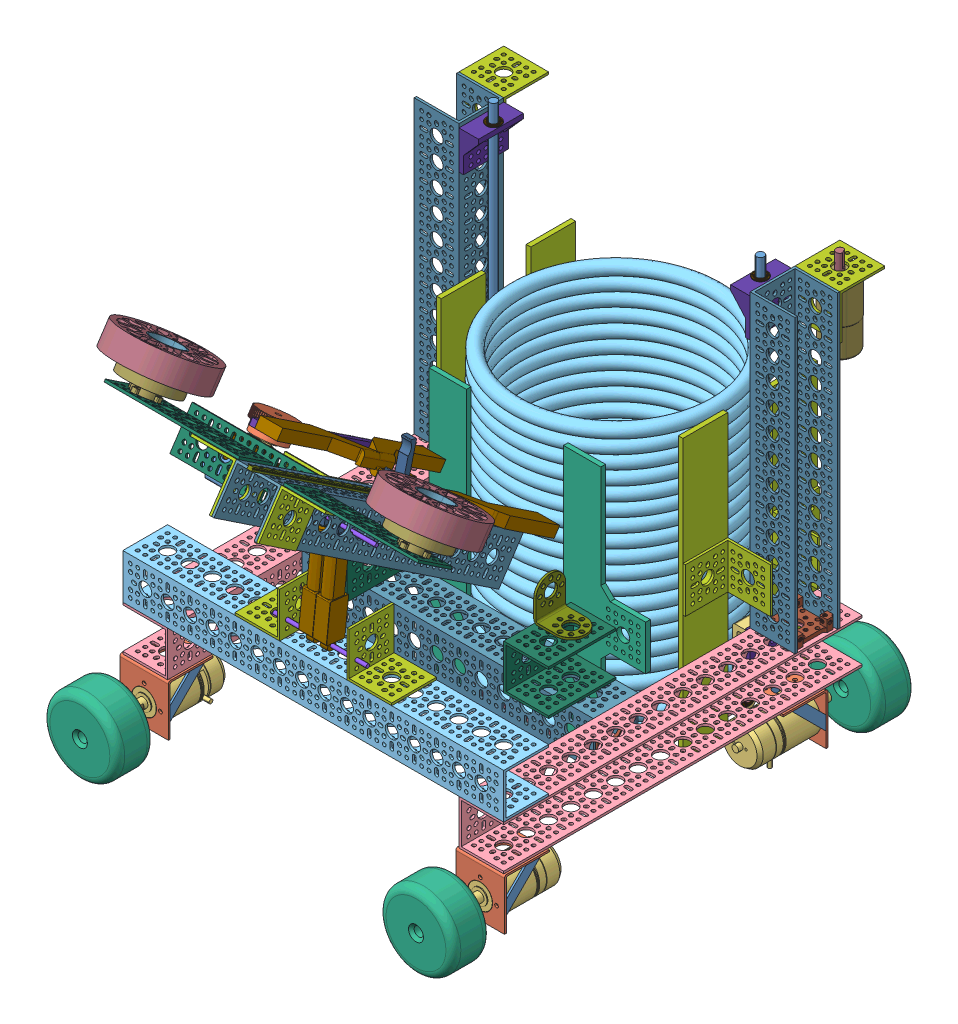
SolidWorks assembly 底座3.0, configuration 默认. Lengths in mm.
Overall size (455.34 460.3 601.78).
126 component instances, 39 part files, 217 mates.
Components (placement in the parent):
- 电机连接支架-5: 电机连接支架 [默认] at (-222.052 128.3372 691.3695) x (0 0 1) z (-1 0 0) size (48 54.5 52)
  - 小兔电机连接支架02-1: 小兔电机连接支架02 [默认] at (-18.8303 11.0829 24.6066) size (36.21 36.21 2)
  - 小兔电机连接支架02-2: 小兔电机连接支架02 [默认] at (-18.8303 11.0829 -25.3934) size (36.21 36.21 2)
  - 小兔电机连接支架-1: 小兔电机连接支架 [默认] at (17.3829 -18.9171 0.6066) size (48 54.5 52)
- 电机连接支架-6: 电机连接支架 [默认] at (137.948 128.3372 691.3695) x (0 0 1) z (-1 0 0) size (48 54.5 52)
  - 小兔电机连接支架02-1: 小兔电机连接支架02 [默认] at (-18.8303 11.0829 24.6066) size (36.21 36.21 2)
  - 小兔电机连接支架02-2: 小兔电机连接支架02 [默认] at (-18.8303 11.0829 -25.3934) size (36.21 36.21 2)
  - 小兔电机连接支架-1: 小兔电机连接支架 [默认] at (17.3829 -18.9171 0.6066) size (48 54.5 52)
- 3508无刷电机带减速箱（00）-5: 3508无刷电机带减速箱（00） [默认] at (137.3414 109.4201 681.1524) x (-1 0 0) z (0 -1 0) size (42 98.3 47)
- 3508无刷电机带减速箱（00）-7: 3508无刷电机带减速箱（00） [默认] at (-222.6586 109.4201 681.1524) x (0 -1 0) z (1 0 0) size (42 98.3 47)
- 384mm-U型梁-1: 384mm-U型梁 [默认] at (-201.1586 165.4201 709.5024) x (0 -1 0) z (1 0 0) size (48 384 48)
- 384mm-U型梁-2: 384mm-U型梁 [默认] at (115.8414 165.4201 709.5024) x (0 1 0) z (-1 0 0) size (48 384 48)
- 408mm-U型梁-10: 408mm-U型梁 [默认] at (161.3414 213.4201 707.0024) x (0 1 0) z (0 0 1) size (48 408 48)
- 电机连接支架-7: 电机连接支架 [默认] at (136.7348 128.3372 383.6353) x (0 0 -1) z (1 0 0) size (48 54.5 52)
  - 小兔电机连接支架02-1: 小兔电机连接支架02 [默认] at (-18.8303 11.0829 24.6066) size (36.21 36.21 2)
  - 小兔电机连接支架02-2: 小兔电机连接支架02 [默认] at (-18.8303 11.0829 -25.3934) size (36.21 36.21 2)
  - 小兔电机连接支架-1: 小兔电机连接支架 [默认] at (17.3829 -18.9171 0.6066) size (48 54.5 52)
- 3508无刷电机带减速箱（00）-8: 3508无刷电机带减速箱（00） [默认] at (137.3414 109.4201 393.8524) x (1 0 0) z (0 -1 0) size (42 98.3 47)
- 电机连接支架-8: 电机连接支架 [默认] at (-223.2652 128.3372 383.6353) x (0 0 -1) z (1 0 0) size (48 54.5 52)
  - 小兔电机连接支架02-1: 小兔电机连接支架02 [默认] at (-18.8303 11.0829 24.6066) size (36.21 36.21 2)
  - 小兔电机连接支架02-2: 小兔电机连接支架02 [默认] at (-18.8303 11.0829 -25.3934) size (36.21 36.21 2)
  - 小兔电机连接支架-1: 小兔电机连接支架 [默认] at (17.3829 -18.9171 0.6066) size (48 54.5 52)
- 3508无刷电机带减速箱（00）-9: 3508无刷电机带减速箱（00） [默认] at (-222.6586 109.4201 393.8524) x (1 0 0) z (0 -1 0) size (42 98.3 47)
- 麦轮（临时）-1: 麦轮（临时） [默认] at (-222.6586 109.4201 324.5024) x (0 0 -1) z (0.996866 -0.079106 0) size (40 80 80)
- 麦轮（临时）-2: 麦轮（临时） [默认] at (137.3414 109.4201 324.5024) x (0 0 -1) z (0.923265 -0.384164 0) size (40 80 80)
- 麦轮（临时）-3: 麦轮（临时） [默认] at (137.3414 109.4201 779.5024) x (0 0 -1) z (0.99707 -0.076496 0) size (40 80 80)
- 麦轮（临时）-4: 麦轮（临时） [默认] at (-222.6586 109.4201 779.5024) x (0 0 -1) z (0.996866 -0.079106 0) size (40 80 80)
- 48x48-L形支架-3: 48x48-L形支架 [默认] at (-81.1586 261.4201 709.5024) x (0 -1 0) z (1 0 0) size (48 48 48)
- 48x48-L形支架-4: 48x48-L形支架 [默认] at (-4.1586 261.4201 661.5024) x (0 -1 0) z (-1 0 0) size (48 48 48)
- 升降轴-1: 升降轴 [默认] at (-92.6586 252.9349 701.0171) x (1 0 0) z (0 0.719401 -0.694595) size (100 4 4)
- 电动推杆01-1: 电动推杆01 [默认] at (-54.1586 252.9349 701.0171) x (1 0 0) z (0 -0.993977 0.109585) size (15 20 103)
- 电动推杆01-2: 电动推杆01 [默认] at (-39.1586 252.9349 701.0171) x (1 0 0) z (0 -0.993977 0.109585) size (15 20 103)
- 电动推杆2-1: 电动推杆2 [默认] at (-35.1586 296.9987 696.1591) x (-1 0 0) z (0 -0.109585 -0.993977) size (9 66 9)
- 电动推杆2-2: 电动推杆2 [默认] at (-50.1586 296.9987 696.1591) x (-1 0 0) z (0 -0.109585 -0.993977) size (9 66 9)
- 升降轴-2: 升降轴 [默认] at (-94.6586 358.1283 689.4197) x (1 0 0) z (0 -0.677442 -0.735576) size (100 4 4)
- 电机转向座-9: 电机转向座 [默认] at (137.3414 189.4201 373.5024) x (0 0 -1) z (1 0 0) size (43.24 12.23 43.24)
- 电机转向座-12: 电机转向座 [默认] at (-222.6586 189.4201 373.5024) x (0 0 -1) z (1 0 0) size (43.24 12.23 43.24)
- 48x48-L形支架-17: 48x48-L形支架 [默认] at (161.3414 477.4201 347.0024) x (0 1 0) z (0 0 1) size (48 48 48)
- 48x48-L形支架-18: 48x48-L形支架 [默认] at (-198.6586 477.4201 347.0024) x (0 1 0) z (0 0 1) size (48 48 48)
- 一级摩擦轮电机01-2: 一级摩擦轮电机01 [默认] at (137.3414 425.6201 325.5024) x (0.035714 0 0.999362) z (-0.999362 0 0.035714) size (36 73.3 36)
- 一级摩擦轮电机02-2: 一级摩擦轮电机02 [默认] at (137.3414 495.9201 325.5024) x (0.907269 0 -0.420551) z (0.420551 0 0.907269) size (8 20 8)
- 312mm-U型梁-7: 312mm-U型梁 [默认] at (-198.6586 186.9201 541.5024) x (0 0 1) z (0 1 0) size (48 312 48)
- 电机转向座-13: 电机转向座 [默认] at (113.3414 165.4201 541.5024) x (0 0 -1) z (0 1 0) size (43.24 12.23 43.24)
- 72mm-U型梁-5: 72mm-U型梁 [默认] at (43.8414 213.4201 517.5024) x (0 -1 0) z (-1 0 0) size (48 72 48)
- 72mm-U型梁-6: 72mm-U型梁 [默认] at (-129.1586 213.4201 517.5024) x (0 1 0) z (1 0 0) size (48 72 48)
- 圆角90°法兰-7: 圆角90°法兰 [默认] at (41.3414 237.4201 541.5024) x (1 0 0) z (0 -1 0) size (40 32 40)
- 圆角90°法兰-8: 圆角90°法兰 [默认] at (-126.6586 237.4201 541.5024) x (-1 0 0) z (0 -1 0) size (40 32 40)
- 轴承座-1: 轴承座 [Default] at (113.3414 492.4201 397.5024) x (-1 0 0) z (0 0 -1) size (21 41 48)
- 8-14轴承-7: 8-14轴承 [默认] at (100.3414 493.4201 373.5024) x (0.974446 0 0.224624) z (-0.224624 0 0.974446) size (15 5 15)
- 轴承座-2: 轴承座 [Default] at (113.3414 150.4201 349.5024) x (-1 0 0) z (0 0 1) size (21 41 48)
- 8-14轴承-8: 8-14轴承 [默认] at (100.3414 146.4201 373.5024) x (0.983901 0 0.178713) z (-0.178713 0 0.983901) size (15 5 15)
- 螺纹杆-3: 螺纹杆 [默认] at (100.3414 117.4201 373.5024) x (0.005803 0 0.999983) z (-0.999983 0 0.005803) size (8 400 8)
- 切边螺纹滑块-1: 切边螺纹滑块 [Default] at (100.3414 178.1581 373.5024) x (-1 0 0) z (0 0 1) size (10.2 15 22)
- 轴承座-3: 轴承座 [Default] at (-198.6586 492.4201 349.5024) size (21 41 48)
- 轴承座-4: 轴承座 [Default] at (-198.6586 150.4201 397.5024) x (1 0 0) z (0 0 -1) size (21 41 48)
- 8-14轴承-9: 8-14轴承 [默认] at (-185.6586 493.4201 373.5024) size (15 5 15)
- 8-14轴承-10: 8-14轴承 [默认] at (-185.6586 146.4201 373.5024) size (15 5 15)
- 螺纹杆-4: 螺纹杆 [默认] at (-185.6586 117.4201 373.5024) x (0.186577 0 0.98244) z (-0.98244 0 0.186577) size (8 400 8)
- 切边螺纹滑块-2: 切边螺纹滑块 [Default] at (-185.6586 178.1581 373.5024) x (-1 0 0) z (0 0 1) size (10.2 15 22)
- 转换块-1: 转换块 [Default] at (100.3414 168.1581 373.5024) x (0 0 1) z (-1 0 0) size (24 85 26)
- 转换块-2: 转换块 [Default] at (-185.6586 168.1581 373.5024) x (0 0 -1) z (1 0 0) size (24 85 26)
- 312mm-U型梁-8: 312mm-U型梁 [默认] at (115.8414 501.4201 373.5024) x (0 0 -1) z (-1 0 0) size (48 312 48)
- 312mm-U型梁-9: 312mm-U型梁 [默认] at (-201.1586 501.4201 373.5024) x (0 0 1) z (1 0 0) size (48 312 48)
- 8-14轴承-11: 8-14轴承 [默认] at (83.3414 100.1581 373.5024) x (0 0.99609 -0.088349) z (0 -0.088349 -0.99609) size (15 5 15)
- 8-14轴承-12: 8-14轴承 [默认] at (-168.6586 100.1581 373.5024) x (0 -0.55352 0.832836) z (0 -0.832836 -0.55352) size (15 5 15)
- 铲板-1: 铲板 [Default] at (-42.6586 84.9017 398.3468) x (-1 0 0) z (0 0.010285 -0.999947) size (262 29 178.51)
- 20个环-3: 20个环 [Default] at (-127.5441 -59.6219 226.4779) size (229.8 290.93 229.39)
  - 圆环-1: 圆环 [默认] at (-22.7884 145.7519 157.2951) size (228 14 228)
  - 圆环-2: 圆环 [默认] at (-23.1175 159.9955 157.1344) size (228 14 228)
  - 圆环-3: 圆环 [默认] at (-23.0314 188.5505 156.9811) size (228 14 228)
  - 圆环-4: 圆环 [默认] at (-22.9968 174.3685 156.6405) size (228 14 228)
  - 圆环-5: 圆环 [默认] at (-23.8175 218.055 156.8293) size (228 14 228)
  - 圆环-6: 圆环 [默认] at (-23.491 232.7117 157.4697) size (228 14 228)
  - 圆环-7: 圆环 [默认] at (-24.5846 203.4176 157.6394) size (228 14 228)
  - 圆环-8: 圆环 [默认] at (-22.9081 247.4608 157.3208) size (228 14 228)
  - 圆环-9: 圆环 [默认] at (-23.5661 364.5462 157.293) size (228 14 228)
  - 圆环-10: 圆环 [默认] at (-23.6099 320.9711 157.4866) size (228 14 228)
  - 圆环-11: 圆环 [默认] at (-23.6825 350.1705 157.5218) size (228 14 228)
  - 圆环-12: 圆环 [默认] at (-24.0088 276.7124 157.1259) size (228 14 228)
  - 圆环-13: 圆环 [默认] at (-23.8881 291.321 157.9228) size (228 14 228)
  - 圆环-14: 圆环 [默认] at (-23.6797 261.8797 158.031) size (228 14 228)
  - 圆环-15: 圆环 [默认] at (-24.0091 335.4434 157.9465) size (228 14 228)
  - 圆环-16: 圆环 [默认] at (-23.4562 306.0805 156.7976) size (228 14 228)
  - 圆环-17: 圆环 [默认] at (-24.0369 393.8042 157.2623) size (228 14 228)
  - 圆环-18: 圆环 [默认] at (-23.9162 408.195 157.1866) size (228 14 228)
  - 圆环-19: 圆环 [默认] at (-23.9606 379.2206 157.4915) size (228 14 228)
  - 圆环-20: 圆环 [默认] at (-23.698 422.6814 157.0029) size (228 14 228)
- 前挡板-1: 前挡板 [Default] at (-94.6586 354.9201 493.5024) x (-1 0 0) z (0 0 -1) size (88 278 5)
- 48x48-L形支架-22: 48x48-L形支架 [默认] at (-198.6586 261.4201 400.0024) x (1 0 0) z (0 0 -1) size (48 48 48)
- 48x48-L形支架-23: 48x48-L形支架 [默认] at (-198.6586 213.4201 347.0024) size (48 48 48)
- 侧挡板-1: 侧挡板 [Default] at (-174.6586 77.4201 301.5024) x (0 0 1) z (1 0 0) size (48 300 5)
- 侧挡板-2: 侧挡板 [Default] at (-174.6586 77.4201 397.5024) x (0 0 1) z (1 0 0) size (48 300 5)
- 侧挡板-3: 侧挡板 [Default] at (84.3414 77.4201 301.5024) x (0 0 1) z (1 0 0) size (48 300 5)
- 侧挡板-4: 侧挡板 [Default] at (84.3414 77.4201 397.5024) x (0 0 1) z (1 0 0) size (48 300 5)
- 48x48-L形支架-24: 48x48-L形支架 [默认] at (91.8414 213.4201 325.5024) x (0 0 1) z (-1 0 0) size (48 48 48)
- 48x48-L形支架-25: 48x48-L形支架 [默认] at (113.3414 213.4201 400.0024) x (-1 0 0) z (0 0 -1) size (48 48 48)
- 前挡板-2: 前挡板 [Default] at (9.3414 354.9201 488.5024) size (88 278 5)
- 蜘蛛钩子-1: 蜘蛛钩子 [默认] at (-41.3293 352.4787 629.0563) x (-1 0 0) z (0 -0.555042 -0.831822) size (146 51.58 210)
  - 滑块1-1: 滑块1 [默认] at (1.3294 2.8515 16) size (12 5 16)
  - 滑块座1-1: 滑块座1 [默认] at (-33.6706 2.8515 4) size (146 18 210)
  - 抓钩1-1: 抓钩1 [默认] at (6.3294 45.8627 -7.2454) x (0 -0.424487 0.905434) z (0 -0.905434 -0.424487) size (35.49 30 38.32)
- 312mm-U型梁-10: 312mm-U型梁 [默认] at (-42.6586 265.9833 509.6053) x (-1 0 0) z (0 0.831822 -0.555042) size (48 312 48)
- 发射法兰1-1: 发射法兰1 [默认] at (-186.6586 457.2783 728.1895) x (-0.530449 -0.470518 -0.70515) z (-0.847717 0.294422 0.44124) size (30 11 30)
- 发射无刷电机-1: 发射无刷电机 [默认] at (-186.6586 429.9945 746.3949) x (0 -0.555042 -0.831822) z (1 0 0) size (58.5 35.4 58.5)
- 摩擦轮-1: 摩擦轮 [默认] at (-186.112 443.4895 719.7023) x (0.95222 -0.169517 -0.25405) z (0 -0.831822 0.555042) size (96 96 24)
  - 摩擦轮.STEP-1: 摩擦轮.STEP [默认] at origin size (96 96 24)
    - 3613-0014-0096 Rubber.STEP-1: 3613-0014-0096 Rubber.STEP [默认] at (-5.0141 13.8433 -6.759) size (96 96 24)
    - 3613-0014-0096 Core.STEP-1: 3613-0014-0096 Core.STEP [默认] at (-5.0141 13.8433 -6.759) x (1 0 0) z (0 -1 0) size (35.2 24 35.2)
- 5孔平板-1: 5孔平板 [默认] at (-210.6586 435.9453 716.5773) x (0 0.831822 -0.555042) z (0 -0.555042 -0.831822) size (2.5 144 43)
- 48x48-L形支架-28: 48x48-L形支架 [默认] at (-69.1586 394.6302 741.1398) x (0 0.831822 -0.555042) z (1 0 0) size (48 48 48)
- 发射法兰1-2: 发射法兰1 [默认] at (101.3414 457.2783 728.1895) x (-0.486014 -0.485079 -0.726972) z (-0.873951 0.269758 0.404277) size (30 11 30)
- 发射无刷电机-2: 发射无刷电机 [默认] at (101.3414 429.9945 746.3949) x (0 0.555042 0.831822) z (-1 0 0) size (58.5 35.4 58.5)
- 摩擦轮-2: 摩擦轮 [默认] at (100.7948 459.8224 744.1798) x (-0.95222 0.169517 0.25405) z (0 -0.831822 0.555042) size (96 96 24)
  - 摩擦轮.STEP-1: 摩擦轮.STEP [默认] at origin size (96 96 24)
    - 3613-0014-0096 Rubber.STEP-1: 3613-0014-0096 Rubber.STEP [默认] at (-5.0141 13.8433 -6.759) size (96 96 24)
    - 3613-0014-0096 Core.STEP-1: 3613-0014-0096 Core.STEP [默认] at (-5.0141 13.8433 -6.759) x (1 0 0) z (0 -1 0) size (35.2 24 35.2)
- 5孔平板-2: 5孔平板 [默认] at (125.3414 459.8121 752.3457) x (0 0.831822 -0.555042) z (0 0.555042 0.831822) size (2.5 144 43)
- 48x48-L形支架-29: 48x48-L形支架 [默认] at (-16.1586 421.2722 781.0673) x (0 0.831822 -0.555042) z (-1 0 0) size (48 48 48)
- 滑轨9-1: 滑轨9 [默认] at (-45.1586 493.584 846.1985) x (1 0 0) z (0 0.555042 0.831822) size (73.65 3.7 429.69)
- 齿条(1)-1: 齿条(1) [默认] at (-115.6586 355.6063 610.1389) x (0 0.555042 0.831822) z (0 -0.831822 0.555042) size (210 7.5 6.5)
- 舵机-1: 舵机 [默认] at (-153.6215 361.5369 660.3751) x (-1 0 0) z (0 0.831822 -0.555042) size (54.3 20 43.9)
- 多功能舵机支架(1)-1: 多功能舵机支架(1) [默认] at (-153.6215 348.9276 685.0784) x (-1 0 0) z (0 -0.555042 -0.831822) size (58 37 25)
- 48x48-L形支架-27: 48x48-L形支架 [默认] at (-90.6586 333.3158 692.49) x (1 0 0) z (0 0.555042 0.831822) size (48 48 48)
- 齿轮(5.23)-1: 齿轮(5.23) [默认] at (-143.7715 383.3306 645.833) x (0.847804 0.294344 0.441124) z (0.53031 -0.470567 -0.705222) size (42 20 42)
- 舵盘(5.23-1: 舵盘(5.23 [默认] at (-143.7715 366.6942 656.9339) x (0.772611 0.352385 0.528107) z (0.63488 -0.428831 -0.642675) size (20 4.78 20)
- 5孔平板-3: 5孔平板 [默认] at (-210.6586 385.8724 689.2789) x (0 0.555042 0.831822) z (0 0.831822 -0.555042) size (2.5 144 43)
Mates (geometry in assembly coordinates):
- Coincident37: coincident anti-aligned: plane of 电机连接支架-5/小兔电机连接支架-1 through (-222.6586 109.4201 708.7524) normal (0 0 -1); plane of 3508无刷电机带减速箱（00）-7 through (-222.6586 96.4201 708.7524) normal (0 0 1)
- Concentric38: concentric aligned: cylinder of 电机连接支架-5/小兔电机连接支架-1 through (-222.6586 109.4201 710.7524) axis (0 0 -1) radius 13.25; cylinder of 3508无刷电机带减速箱（00）-7 through (-222.6586 109.4201 672.4524) axis (0 0 -1) radius 13
- Concentric39: concentric anti-aligned: cylinder of 电机连接支架-5/小兔电机连接支架-1 through (-222.6586 126.9201 710.7524) axis (0 0 -1) radius 2; cylinder of 3508无刷电机带减速箱（00）-7 through (-222.6586 126.9201 708.7524) axis (0 0 1) radius 1.65
- Coincident38: coincident anti-aligned: plane of 电机连接支架-6/小兔电机连接支架-1 through (137.3414 109.4201 708.7524) normal (0 0 -1); plane of 3508无刷电机带减速箱（00）-5 through (124.3414 109.4201 708.7524) normal (0 0 1)
- Concentric40: concentric aligned: cylinder of 电机连接支架-6/小兔电机连接支架-1 through (137.3414 109.4201 710.7524) axis (0 0 -1) radius 13.25; cylinder of 3508无刷电机带减速箱（00）-5 through (137.3414 109.4201 672.4524) axis (0 0 -1) radius 13
- Concentric41: concentric anti-aligned: cylinder of 电机连接支架-6/小兔电机连接支架-1 through (137.3414 126.9201 710.7524) axis (0 0 -1) radius 2; cylinder of 3508无刷电机带减速箱（00）-5 through (137.3414 126.9201 708.7524) axis (0 0 1) radius 1.65
- Concentric261: concentric anti-aligned: cylinder of 384mm-U型梁-2 through (137.3414 179.4201 685.5024) axis (0 1 0) radius 7; cylinder of 408mm-U型梁-10 through (137.3414 199.4201 685.5024) axis (0 -1 0) radius 7
- Concentric262: concentric anti-aligned: cylinder of 384mm-U型梁-1 through (-222.6586 179.4201 685.5024) axis (0 1 0) radius 7; cylinder of 408mm-U型梁-10 through (-222.6586 199.4201 685.5024) axis (0 -1 0) radius 7
- Coincident94: coincident aligned: plane of 384mm-U型梁-2 through (161.3414 186.9201 325.5024) normal (1 0 0); plane of 408mm-U型梁-10 through (161.3414 213.4201 707.0024) normal (1 0 0)
- Coincident95: coincident aligned: plane of 384mm-U型梁-1 through (-246.6586 186.9201 325.5024) normal (-1 0 0); plane of 408mm-U型梁-10 through (-246.6586 213.4201 707.0024) normal (-1 0 0)
- Coincident96: coincident anti-aligned: plane of 384mm-U型梁-1 through (-246.6586 189.4201 325.5024) normal (0 1 0); plane of 408mm-U型梁-10 through (-246.6586 189.4201 661.5024) normal (0 -1 0)
- Coincident97: coincident anti-aligned: plane of 384mm-U型梁-2 through (161.3414 189.4201 325.5024) normal (0 1 0); plane of 408mm-U型梁-10 through (-246.6586 189.4201 661.5024) normal (0 -1 0)
- Concentric267: concentric aligned: cylinder of 电机连接支架-7/小兔电机连接支架-1 through (137.3414 109.4201 364.2524) axis (0 0 1) radius 13.25; cylinder of 3508无刷电机带减速箱（00）-8 through (137.3414 109.4201 402.5524) axis (0 0 1) radius 13
- Coincident104: coincident anti-aligned: plane of 电机连接支架-7/小兔电机连接支架-1 through (137.3414 109.4201 366.2524) normal (0 0 1); plane of 3508无刷电机带减速箱（00）-8 through (150.3414 109.4201 366.2524) normal (0 0 -1)
- Concentric268: concentric anti-aligned: cylinder of 电机连接支架-7/小兔电机连接支架-1 through (137.3414 126.9201 364.2524) axis (0 0 1) radius 2; cylinder of 3508无刷电机带减速箱（00）-8 through (137.3414 126.9201 366.2524) axis (0 0 -1) radius 1.65
- Concentric269: concentric aligned: cylinder of 电机连接支架-8/小兔电机连接支架-1 through (-222.6586 109.4201 364.2524) axis (0 0 1) radius 13.25; cylinder of 3508无刷电机带减速箱（00）-9 through (-222.6586 109.4201 402.5524) axis (0 0 1) radius 13
- Coincident105: coincident anti-aligned: plane of 电机连接支架-8/小兔电机连接支架-1 through (-222.6586 109.4201 366.2524) normal (0 0 1); plane of 3508无刷电机带减速箱（00）-9 through (-209.6586 109.4201 366.2524) normal (0 0 -1)
- Concentric270: concentric anti-aligned: cylinder of 电机连接支架-8/小兔电机连接支架-1 through (-222.6586 126.9201 364.2524) axis (0 0 1) radius 2; cylinder of 3508无刷电机带减速箱（00）-9 through (-222.6586 126.9201 366.2524) axis (0 0 -1) radius 1.65
- Concentric271: concentric anti-aligned: cylinder of 电机连接支架-6/小兔电机连接支架-1 through (137.3414 86.9201 685.5024) axis (0 1 0) radius 7; cylinder of 384mm-U型梁-2 through (137.3414 151.4201 685.5024) axis (0 -1 0) radius 7
- Coincident106: coincident anti-aligned: plane of 电机连接支架-6/小兔电机连接支架-1 through (163.3414 141.4201 662.7524) normal (0 1 0); plane of 384mm-U型梁-2 through (161.3414 141.4201 325.5024) normal (0 -1 0)
- Concentric272: concentric anti-aligned: cylinder of 电机连接支架-6/小兔电机连接支架-1 through (153.3414 86.9201 701.5024) axis (0 1 0) radius 2; cylinder of 384mm-U型梁-2 through (153.3414 151.4201 701.5024) axis (0 -1 0) radius 2
- Concentric273: concentric anti-aligned: cylinder of 电机连接支架-5/小兔电机连接支架-1 through (-222.6586 86.9201 685.5024) axis (0 1 0) radius 7; cylinder of 384mm-U型梁-1 through (-222.6586 151.4201 685.5024) axis (0 -1 0) radius 7
- Coincident107: coincident anti-aligned: plane of 电机连接支架-5/小兔电机连接支架-1 through (-196.6586 141.4201 662.7524) normal (0 1 0); plane of 384mm-U型梁-1 through (-246.6586 141.4201 325.5024) normal (0 -1 0)
- Concentric274: concentric anti-aligned: cylinder of 电机连接支架-5/小兔电机连接支架-1 through (-206.6586 86.9201 701.5024) axis (0 1 0) radius 2; cylinder of 384mm-U型梁-1 through (-206.6586 151.4201 701.5024) axis (0 -1 0) radius 2
- Coincident108: coincident anti-aligned: plane of 384mm-U型梁-2 through (161.3414 141.4201 325.5024) normal (0 -1 0); plane of 电机连接支架-7/小兔电机连接支架-1 through (111.3414 141.4201 412.2524) normal (0 1 0)
- Concentric276: concentric anti-aligned: cylinder of 384mm-U型梁-2 through (153.3414 151.4201 373.5024) axis (0 -1 0) radius 2; cylinder of 电机连接支架-7/小兔电机连接支架-1 through (153.3414 86.9201 373.5024) axis (0 1 0) radius 2
- Concentric277: concentric anti-aligned: cylinder of 384mm-U型梁-2 through (121.3414 151.4201 373.5024) axis (0 -1 0) radius 2; cylinder of 电机连接支架-7/小兔电机连接支架-1 through (121.3414 86.9201 373.5024) axis (0 1 0) radius 2
- Coincident109: coincident anti-aligned: plane of 384mm-U型梁-1 through (-246.6586 141.4201 325.5024) normal (0 -1 0); plane of 电机连接支架-8/小兔电机连接支架-1 through (-248.6586 141.4201 412.2524) normal (0 1 0)
- Concentric278: concentric anti-aligned: cylinder of 384mm-U型梁-1 through (-238.6586 151.4201 373.5024) axis (0 -1 0) radius 2; cylinder of 电机连接支架-8/小兔电机连接支架-1 through (-238.6586 86.9201 373.5024) axis (0 1 0) radius 2
- Concentric279: concentric anti-aligned: cylinder of 384mm-U型梁-1 through (-206.6586 151.4201 373.5024) axis (0 -1 0) radius 2; cylinder of 电机连接支架-8/小兔电机连接支架-1 through (-206.6586 86.9201 373.5024) axis (0 1 0) radius 2
- Concentric280: concentric anti-aligned: cylinder of 3508无刷电机带减速箱（00）-9 through (-222.6586 109.4201 402.5524) axis (0 0 1) radius 5; cylinder of 麦轮（临时）-1 through (-222.6586 109.4201 324.5024) axis (0 0 -1) radius 5
- Distance1: distance = 1 mm anti-aligned: plane of 麦轮（临时）-1 through (-222.6586 109.4201 324.5024) normal (0 0 1); plane of 384mm-U型梁-1 through (-201.1586 165.4201 325.5024) normal (0 0 -1)
- Concentric281: concentric anti-aligned: cylinder of 3508无刷电机带减速箱（00）-8 through (137.3414 109.4201 402.5524) axis (0 0 1) radius 5; cylinder of 麦轮（临时）-2 through (137.3414 109.4201 324.5024) axis (0 0 -1) radius 5
- Distance2: distance = 1 mm anti-aligned: plane of 384mm-U型梁-2 through (115.8414 165.4201 325.5024) normal (0 0 -1); plane of 麦轮（临时）-2 through (137.3414 109.4201 324.5024) normal (0 0 1)
- Concentric282: concentric aligned: cylinder of 3508无刷电机带减速箱（00）-5 through (137.3414 109.4201 672.4524) axis (0 0 -1) radius 5; cylinder of 麦轮（临时）-3 through (137.3414 109.4201 779.5024) axis (0 0 -1) radius 5
- Distance3: distance = 495 mm anti-aligned: plane of 麦轮（临时）-3 through (137.3414 109.4201 779.5024) normal (0 0 1); plane of 麦轮（临时）-2 through (137.3414 109.4201 284.5024) normal (0 0 -1)
- Concentric283: concentric aligned: cylinder of 3508无刷电机带减速箱（00）-7 through (-222.6586 109.4201 672.4524) axis (0 0 -1) radius 5; cylinder of 麦轮（临时）-4 through (-222.6586 109.4201 779.5024) axis (0 0 -1) radius 5
- Distance4: distance = 495 mm anti-aligned: plane of 麦轮（临时）-4 through (-222.6586 109.4201 779.5024) normal (0 0 1); plane of 麦轮（临时）-1 through (-222.6586 109.4201 284.5024) normal (0 0 -1)
- Coincident120: coincident anti-aligned: plane of 408mm-U型梁-10 through (-246.6586 237.4201 661.5024) normal (0 1 0); plane of 48x48-L形支架-3 through (-126.6586 237.4201 661.5024) normal (0 -1 0)
- Concentric309: concentric anti-aligned: cylinder of 408mm-U型梁-10 through (-102.6586 227.4201 685.5024) axis (0 1 0) radius 7; cylinder of 48x48-L形支架-3 through (-102.6586 247.4201 685.5024) axis (0 -1 0) radius 7
- Concentric310: concentric anti-aligned: cylinder of 408mm-U型梁-10 through (-118.6586 227.4201 669.5024) axis (0 1 0) radius 2; cylinder of 48x48-L形支架-3 through (-118.6586 247.4201 669.5024) axis (0 -1 0) radius 2
- Concentric311: concentric anti-aligned: cylinder of 408mm-U型梁-10 through (17.3414 227.4201 685.5024) axis (0 1 0) radius 7; cylinder of 48x48-L形支架-4 through (17.3414 247.4201 685.5024) axis (0 -1 0) radius 7
- Coincident121: coincident anti-aligned: plane of 408mm-U型梁-10 through (-246.6586 237.4201 661.5024) normal (0 1 0); plane of 48x48-L形支架-4 through (41.3414 237.4201 709.5024) normal (0 -1 0)
- Concentric312: concentric anti-aligned: cylinder of 408mm-U型梁-10 through (1.3414 227.4201 701.5024) axis (0 1 0) radius 2; cylinder of 48x48-L形支架-4 through (1.3414 247.4201 701.5024) axis (0 -1 0) radius 2
- Concentric313: concentric anti-aligned: cylinder of 48x48-L形支架-3 through (-88.6586 252.9349 701.0171) axis (1 0 0) radius 2; cylinder of 升降轴-1 through (7.3414 252.9349 701.0171) axis (-1 0 0) radius 2
- Distance6: distance = 11.5 mm aligned: plane of 升降轴-1 through (-92.6586 252.9349 701.0171) normal (-1 0 0); plane of 48x48-L形支架-3 through (-81.1586 282.9201 661.5024) normal (-1 0 0)
- Concentric323: concentric aligned: cylinder of 升降轴-1 through (7.3414 252.9349 701.0171) axis (-1 0 0) radius 2; cylinder of 电动推杆01-1 through (-46.1586 252.9349 701.0171) axis (-1 0 0) radius 2
- Concentric324: concentric aligned: cylinder of 升降轴-1 through (7.3414 252.9349 701.0171) axis (-1 0 0) radius 2; cylinder of 电动推杆01-2 through (-31.1586 252.9349 701.0171) axis (-1 0 0) radius 2
- Concentric325: concentric anti-aligned: cylinder of 电动推杆01-2 through (-35.1586 296.1729 696.2502) axis (0 0.993977 -0.109585) radius 4.5; cylinder of 电动推杆2-1 through (-35.1586 351.6675 690.132) axis (0 -0.993977 0.109585) radius 4.5
- LimitDistance1: limit distance = 54.1692 mm anti-aligned: plane of 电动推杆2-1 through (-35.1586 296.9987 696.1591) normal (0 -0.993977 0.109585); plane of 电动推杆01-2 through (-35.1586 350.8416 690.223) normal (0 0.993977 -0.109585)
- LimitDistance2: limit distance = 0.8308 mm aligned: plane of 电动推杆2-1 through (-35.1586 351.6675 690.132) normal (0 0.993977 -0.109585); plane of 电动推杆01-2 through (-35.1586 350.8416 690.223) normal (0 0.993977 -0.109585)
- Concentric328: concentric anti-aligned: cylinder of 电动推杆01-1 through (-50.1586 296.1729 696.2502) axis (0 0.993977 -0.109585) radius 4.5; cylinder of 电动推杆2-2 through (-50.1586 351.6675 690.132) axis (0 -0.993977 0.109585) radius 4.5
- LimitDistance6: limit distance = 54.1692 mm anti-aligned: plane of 电动推杆01-1 through (-50.1586 350.8416 690.223) normal (0 0.993977 -0.109585); plane of 电动推杆2-2 through (-50.1586 296.9987 696.1591) normal (0 -0.993977 0.109585)
- LimitDistance7: limit distance = 0.8308 mm aligned: plane of 电动推杆2-2 through (-50.1586 351.6675 690.132) normal (0 0.993977 -0.109585); plane of 电动推杆01-1 through (-50.1586 350.8416 690.223) normal (0 0.993977 -0.109585)
- Coincident131: coincident anti-aligned: plane of 电动推杆01-1 through (-42.6586 295.077 686.3104) normal (1 0 0); plane of 电动推杆01-2 through (-42.6586 297.2687 706.19) normal (-1 0 0)
- Distance12: distance = 21 mm anti-aligned: plane of 电动推杆01-1 through (-57.6586 297.2687 706.19) normal (-1 0 0); plane of 48x48-L形支架-3 through (-78.6586 237.4201 661.5024) normal (1 0 0)
- Coincident286: coincident anti-aligned: plane of 384mm-U型梁-2 through (161.3414 189.4201 325.5024) normal (0 1 0); plane of 电机转向座-9 through (137.3414 189.4201 373.5024) normal (0 -1 0)
- Concentric623: concentric anti-aligned: cylinder of 48x48-L形支架-17 through (137.3414 491.4201 325.5024) axis (0 1 0) radius 7; cylinder of 一级摩擦轮电机01-2 through (137.3414 498.9201 325.5024) axis (0 -1 0) radius 11
- Coincident301: coincident anti-aligned: plane of 48x48-L形支架-17 through (113.3414 498.9201 347.0024) normal (0 -1 0); plane of 一级摩擦轮电机01-2 through (137.3414 498.9201 325.5024) normal (0 1 0)
- Tangent10: tangent anti-aligned: plane of 48x48-L形支架-17 through (135.3414 491.4201 347.0024) normal (1 0 0); cylinder of 一级摩擦轮电机01-2 through (136.8414 491.6201 311.5113) axis (0 1 0) radius 1.5
- Concentric624: concentric anti-aligned: cylinder of 一级摩擦轮电机01-2 through (137.3414 495.9201 325.5024) axis (0 1 0) radius 4; cylinder of 一级摩擦轮电机02-2 through (137.3414 515.9201 325.5024) axis (0 -1 0) radius 4
- Coincident302: coincident anti-aligned: plane of 一级摩擦轮电机01-2 through (137.3414 495.9201 325.5024) normal (0 1 0); plane of 一级摩擦轮电机02-2 through (137.3414 495.9201 325.5024) normal (0 -1 0)
- Concentric637: concentric aligned: cylinder of 384mm-U型梁-1 through (-222.6586 179.4201 373.5024) axis (0 1 0) radius 7; cylinder of 电机转向座-12 through (-222.6586 189.4201 373.5024) axis (0 1 0) radius 7
- Concentric638: concentric aligned: cylinder of 384mm-U型梁-2 through (137.3414 179.4201 373.5024) axis (0 1 0) radius 7; cylinder of 电机转向座-9 through (137.3414 189.4201 373.5024) axis (0 1 0) radius 7
- Coincident316: coincident aligned: plane of 384mm-U型梁-2 through (161.3414 189.4201 325.5024) normal (0 1 0); plane of 312mm-U型梁-7 through (113.3414 189.4201 565.5024) normal (0 1 0)
- Coincident317: coincident anti-aligned: plane of 384mm-U型梁-2 through (113.3414 189.4201 325.5024) normal (-1 0 0); plane of 312mm-U型梁-7 through (113.3414 186.9201 541.5024) normal (1 0 0)
- Concentric650: concentric anti-aligned: cylinder of 312mm-U型梁-7 through (105.3414 179.4201 557.5024) axis (0 1 0) radius 2; cone of 电机转向座-13 through (105.3414 186.9201 557.5024) axis (0 -1 0)
